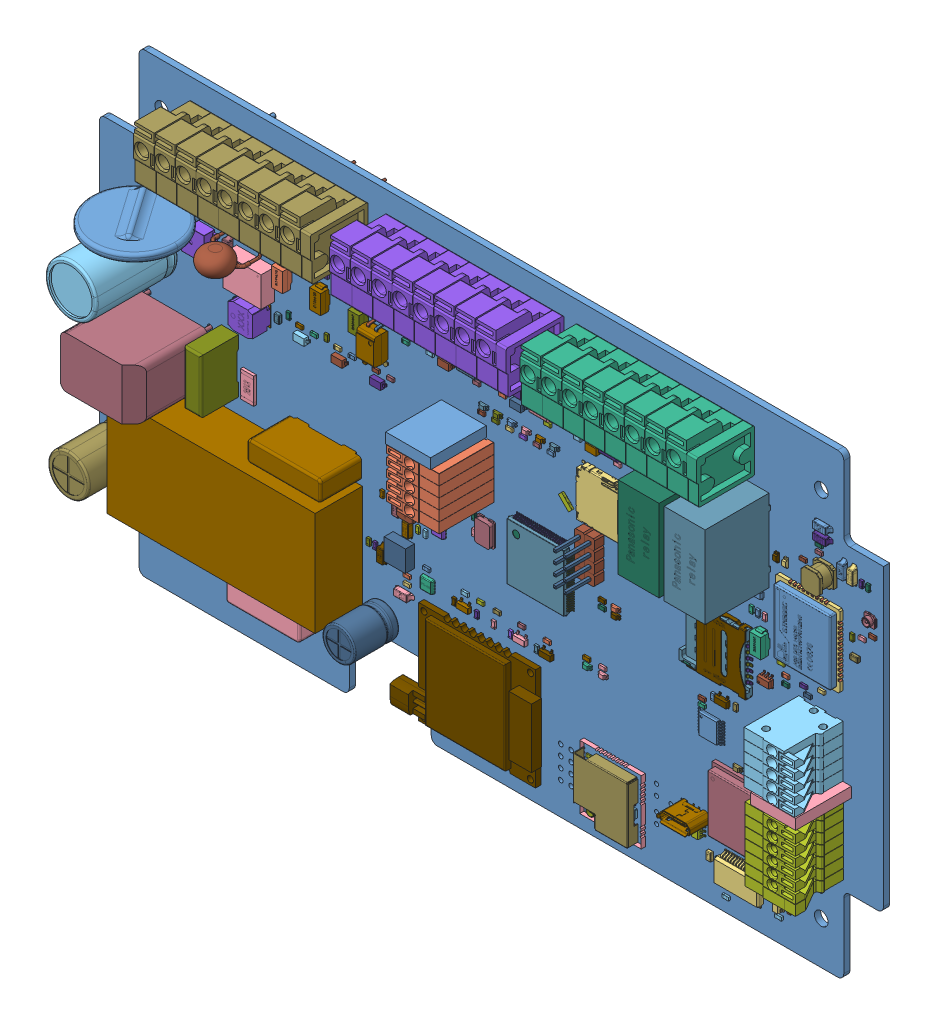
SolidWorks assembly Velvet_Controller_V1.2_2023, configuration Default. Lengths in mm. (continued)
Components (placement in the parent): (continued)
- Velvet_Controller_V1.2_2023(2)^Velvet_Controller_V1.2_2023-1: Velvet_Controller_V1.2_2023(2)^Velvet_Controller_V1.2_2023 [Default] at origin size (191.4 111.4 51.25) (virtual) (continued)
  - DD2lr^Velvet_Controller_V1.2_2023(2)_Velvet_Controller_V1.2_2023-1: DD2lr^Velvet_Controller_V1.2_2023(2)_Velvet_Controller_V1.2_2023 [Default] at origin size (15 15.75 3.52) (virtual) (continued)
    - 3D_RAK3172^DD2lr_Velvet_Controller_V1.2_2023(2)_Velvet_Controller_V1.2_2023-1: 3D_RAK3172^DD2lr_Velvet_Controller_V1.2_2023(2)_Velvet_Controller_V1.2_2023 [Default] at (133.2551 19.6 1) x (-1 0 0) z (0 0 1) size (15 15.75 3.52) (virtual) (continued)
      - C34^3D_RAK3172_DD2lr_Velvet_Controller_V1.2_2023(2)_Velvet_Controller_V1.2_2023-1: C34^3D_RAK3172_DD2lr_Velvet_Controller_V1.2_2023(2)_Velvet_Controller_V1.2_2023 [Default] at origin size (0.3 0.6 0.3) (virtual)
        - 0201_SMD_Capacitor^C34_3D_RAK3172_DD2lr_Velvet_Controller_V1.2_2023(2)_Velvet_Controller_V1.2_2023-1: 0201_SMD_Capacitor^C34_3D_RAK3172_DD2lr_Velvet_Controller_V1.2_2023(2)_Velvet_Controller_V1.2_2023 [Default] at (4.318 4.2211 0.2794) x (0 1 0) z (0 0 1) size (0.6 0.3 0.3) (virtual)
      - C35^3D_RAK3172_DD2lr_Velvet_Controller_V1.2_2023(2)_Velvet_Controller_V1.2_2023-1: C35^3D_RAK3172_DD2lr_Velvet_Controller_V1.2_2023(2)_Velvet_Controller_V1.2_2023 [Default] at origin size (0.6 0.3 0.3) (virtual)
        - 0201_SMD_Capacitor^C35_3D_RAK3172_DD2lr_Velvet_Controller_V1.2_2023(2)_Velvet_Controller_V1.2_2023-1: 0201_SMD_Capacitor^C35_3D_RAK3172_DD2lr_Velvet_Controller_V1.2_2023(2)_Velvet_Controller_V1.2_2023 [Default] at (9.0365 2.3622 0.2794) x (1 0 0) z (0 0 1) size (0.6 0.3 0.3) (virtual)
      - C36^3D_RAK3172_DD2lr_Velvet_Controller_V1.2_2023(2)_Velvet_Controller_V1.2_2023-1: C36^3D_RAK3172_DD2lr_Velvet_Controller_V1.2_2023(2)_Velvet_Controller_V1.2_2023 [Default] at origin size (0.3 0.6 0.3) (virtual)
        - 0201_SMD_Capacitor^C36_3D_RAK3172_DD2lr_Velvet_Controller_V1.2_2023(2)_Velvet_Controller_V1.2_2023-1: 0201_SMD_Capacitor^C36_3D_RAK3172_DD2lr_Velvet_Controller_V1.2_2023(2)_Velvet_Controller_V1.2_2023 [Default] at (13.0302 10.0751 0.2794) x (0 -1 0) z (0 0 1) size (0.6 0.3 0.3) (virtual)
      - C37^3D_RAK3172_DD2lr_Velvet_Controller_V1.2_2023(2)_Velvet_Controller_V1.2_2023-1: C37^3D_RAK3172_DD2lr_Velvet_Controller_V1.2_2023(2)_Velvet_Controller_V1.2_2023 [Default] at origin size (0.3 0.6 0.3) (virtual)
        - 0201_SMD_Capacitor^C37_3D_RAK3172_DD2lr_Velvet_Controller_V1.2_2023(2)_Velvet_Controller_V1.2_2023-1: 0201_SMD_Capacitor^C37_3D_RAK3172_DD2lr_Velvet_Controller_V1.2_2023(2)_Velvet_Controller_V1.2_2023 [Default] at (3.7338 4.2211 0.2794) x (0 1 0) z (0 0 1) size (0.6 0.3 0.3) (virtual)
      - C38^3D_RAK3172_DD2lr_Velvet_Controller_V1.2_2023(2)_Velvet_Controller_V1.2_2023-1: C38^3D_RAK3172_DD2lr_Velvet_Controller_V1.2_2023(2)_Velvet_Controller_V1.2_2023 [Default] at origin size (1 0.5 0.5) (virtual)
        - C0402^C38_3D_RAK3172_DD2lr_Velvet_Controller_V1.2_2023(2)_Velvet_Controller_V1.2_2023-1: C0402^C38_3D_RAK3172_DD2lr_Velvet_Controller_V1.2_2023(2)_Velvet_Controller_V1.2_2023 [Default] at (2.3114 4.7323 0.254) x (1 0 0) z (0 0 1) size (1 0.5 0.5) (virtual)
      - C39^3D_RAK3172_DD2lr_Velvet_Controller_V1.2_2023(2)_Velvet_Controller_V1.2_2023-1: C39^3D_RAK3172_DD2lr_Velvet_Controller_V1.2_2023(2)_Velvet_Controller_V1.2_2023 [Default] at origin size (0.6 0.3 0.3) (virtual)
        - 0201_SMD_Capacitor^C39_3D_RAK3172_DD2lr_Velvet_Controller_V1.2_2023(2)_Velvet_Controller_V1.2_2023-1: 0201_SMD_Capacitor^C39_3D_RAK3172_DD2lr_Velvet_Controller_V1.2_2023(2)_Velvet_Controller_V1.2_2023 [Default] at (4.0593 3.1881 0.2794) x (-1 0 0) z (0 0 1) size (0.6 0.3 0.3) (virtual)
      - C40^3D_RAK3172_DD2lr_Velvet_Controller_V1.2_2023(2)_Velvet_Controller_V1.2_2023-1: C40^3D_RAK3172_DD2lr_Velvet_Controller_V1.2_2023(2)_Velvet_Controller_V1.2_2023 [Default] at origin size (0.3 0.6 0.3) (virtual)
        - 0201_SMD_Capacitor^C40_3D_RAK3172_DD2lr_Velvet_Controller_V1.2_2023(2)_Velvet_Controller_V1.2_2023-1: 0201_SMD_Capacitor^C40_3D_RAK3172_DD2lr_Velvet_Controller_V1.2_2023(2)_Velvet_Controller_V1.2_2023 [Default] at (3.6576 1.7319 0.2794) x (0 1 0) z (0 0 1) size (0.6 0.3 0.3) (virtual)
      - L1^3D_RAK3172_DD2lr_Velvet_Controller_V1.2_2023(2)_Velvet_Controller_V1.2_2023-1: L1^3D_RAK3172_DD2lr_Velvet_Controller_V1.2_2023(2)_Velvet_Controller_V1.2_2023 [Default] at origin size (0.68 0.33 0.34) (virtual)
        - R0201^L1_3D_RAK3172_DD2lr_Velvet_Controller_V1.2_2023(2)_Velvet_Controller_V1.2_2023-1: R0201^L1_3D_RAK3172_DD2lr_Velvet_Controller_V1.2_2023(2)_Velvet_Controller_V1.2_2023 [Default] at (7.8526 11.2014 0) x (-1 0 0) z (0 1 0) size (0.68 0.34 0.33) (virtual)
      - L3^3D_RAK3172_DD2lr_Velvet_Controller_V1.2_2023(2)_Velvet_Controller_V1.2_2023-1: L3^3D_RAK3172_DD2lr_Velvet_Controller_V1.2_2023(2)_Velvet_Controller_V1.2_2023 [Default] at origin size (0.33 0.68 0.34) (virtual)
        - R0201^L3_3D_RAK3172_DD2lr_Velvet_Controller_V1.2_2023(2)_Velvet_Controller_V1.2_2023-1: R0201^L3_3D_RAK3172_DD2lr_Velvet_Controller_V1.2_2023(2)_Velvet_Controller_V1.2_2023 [Default] at (1.7272 13.1318 0) x (0 -1 0) z (-1 0 0) size (0.68 0.34 0.33) (virtual)
      - L5^3D_RAK3172_DD2lr_Velvet_Controller_V1.2_2023(2)_Velvet_Controller_V1.2_2023-1: L5^3D_RAK3172_DD2lr_Velvet_Controller_V1.2_2023(2)_Velvet_Controller_V1.2_2023 [Default] at origin size (0.68 0.33 0.34) (virtual)
        - R0201^L5_3D_RAK3172_DD2lr_Velvet_Controller_V1.2_2023(2)_Velvet_Controller_V1.2_2023-1: R0201^L5_3D_RAK3172_DD2lr_Velvet_Controller_V1.2_2023(2)_Velvet_Controller_V1.2_2023 [Default] at (8.0772 13.3096 0) x (-1 0 0) z (0 1 0) size (0.68 0.34 0.33) (virtual)
      - L6^3D_RAK3172_DD2lr_Velvet_Controller_V1.2_2023(2)_Velvet_Controller_V1.2_2023-1: L6^3D_RAK3172_DD2lr_Velvet_Controller_V1.2_2023(2)_Velvet_Controller_V1.2_2023 [Default] at origin size (1 0.5 0.5) (virtual)
        - C0402^L6_3D_RAK3172_DD2lr_Velvet_Controller_V1.2_2023(2)_Velvet_Controller_V1.2_2023-1: C0402^L6_3D_RAK3172_DD2lr_Velvet_Controller_V1.2_2023(2)_Velvet_Controller_V1.2_2023 [Default] at (5.822 11.0823 0.254) x (1 0 0) z (0 0 1) size (1 0.5 0.5) (virtual)
      - L7^3D_RAK3172_DD2lr_Velvet_Controller_V1.2_2023(2)_Velvet_Controller_V1.2_2023-1: L7^3D_RAK3172_DD2lr_Velvet_Controller_V1.2_2023(2)_Velvet_Controller_V1.2_2023 [Default] at origin size (0.68 0.33 0.34) (virtual)
        - R0201^L7_3D_RAK3172_DD2lr_Velvet_Controller_V1.2_2023(2)_Velvet_Controller_V1.2_2023-1: R0201^L7_3D_RAK3172_DD2lr_Velvet_Controller_V1.2_2023(2)_Velvet_Controller_V1.2_2023 [Default] at (3.5854 12.1158 0) x (1 0 0) z (0 -1 0) size (0.68 0.34 0.33) (virtual)
      - L9^3D_RAK3172_DD2lr_Velvet_Controller_V1.2_2023(2)_Velvet_Controller_V1.2_2023-1: L9^3D_RAK3172_DD2lr_Velvet_Controller_V1.2_2023(2)_Velvet_Controller_V1.2_2023 [Default] at origin size (1.15 0.55 0.41) (virtual)
        - RES_1005-0402^L9_3D_RAK3172_DD2lr_Velvet_Controller_V1.2_2023(2)_Velvet_Controller_V1.2_2023-1: RES_1005-0402^L9_3D_RAK3172_DD2lr_Velvet_Controller_V1.2_2023(2)_Velvet_Controller_V1.2_2023 [Default] at (3.9641 11.3538 0) x (-1 0 0) z (0 1 0) size (1.15 0.41 0.55) (virtual)
      - L20^3D_RAK3172_DD2lr_Velvet_Controller_V1.2_2023(2)_Velvet_Controller_V1.2_2023-1: L20^3D_RAK3172_DD2lr_Velvet_Controller_V1.2_2023(2)_Velvet_Controller_V1.2_2023 [Default] at origin size (1.6 0.8 0.3) (virtual)
        - 6559637360^L20_3D_RAK3172_DD2lr_Velvet_Controller_V1.2_2023(2)_Velvet_Controller_V1.2_2023-1: 6559637360^L20_3D_RAK3172_DD2lr_Velvet_Controller_V1.2_2023(2)_Velvet_Controller_V1.2_2023 [Default] at (12.3698 2.0828 0) x (-1 0 0) z (0 1 0) size (1.6 0.3 0.8) (virtual)
      - L30^3D_RAK3172_DD2lr_Velvet_Controller_V1.2_2023(2)_Velvet_Controller_V1.2_2023-1: L30^3D_RAK3172_DD2lr_Velvet_Controller_V1.2_2023(2)_Velvet_Controller_V1.2_2023 [Default] at origin size (1.15 0.55 0.41) (virtual)
        - RES_1005-0402^L30_3D_RAK3172_DD2lr_Velvet_Controller_V1.2_2023(2)_Velvet_Controller_V1.2_2023-1: RES_1005-0402^L30_3D_RAK3172_DD2lr_Velvet_Controller_V1.2_2023(2)_Velvet_Controller_V1.2_2023 [Default] at (7.1263 1.8 0) x (-1 0 0) z (0 1 0) size (1.15 0.41 0.55) (virtual)
      - X2^3D_RAK3172_DD2lr_Velvet_Controller_V1.2_2023(2)_Velvet_Controller_V1.2_2023-1: X2^3D_RAK3172_DD2lr_Velvet_Controller_V1.2_2023(2)_Velvet_Controller_V1.2_2023 [Default] at origin size (1.2 2 0.61) (virtual)
        - crystal_rtf2012^X2_3D_RAK3172_DD2lr_Velvet_Controller_V1.2_2023(2)_Velvet_Controller_V1.2_2023-1: crystal_rtf2012^X2_3D_RAK3172_DD2lr_Velvet_Controller_V1.2_2023(2)_Velvet_Controller_V1.2_2023 [Default] at (2.25 2.8402 0) x (0 1 0) z (1 0 0) size (2 0.61 1.2) (virtual)
      - R2^3D_RAK3172_DD2lr_Velvet_Controller_V1.2_2023(2)_Velvet_Controller_V1.2_2023-1: R2^3D_RAK3172_DD2lr_Velvet_Controller_V1.2_2023(2)_Velvet_Controller_V1.2_2023 [Default] at origin size (0.68 0.33 0.34) (virtual)
        - R0201^R2_3D_RAK3172_DD2lr_Velvet_Controller_V1.2_2023(2)_Velvet_Controller_V1.2_2023-1: R0201^R2_3D_RAK3172_DD2lr_Velvet_Controller_V1.2_2023(2)_Velvet_Controller_V1.2_2023 [Default] at (1.9613 10.1854 0) x (1 0 0) z (0 -1 0) size (0.68 0.34 0.33) (virtual)
      - C5^3D_RAK3172_DD2lr_Velvet_Controller_V1.2_2023(2)_Velvet_Controller_V1.2_2023-1: C5^3D_RAK3172_DD2lr_Velvet_Controller_V1.2_2023(2)_Velvet_Controller_V1.2_2023 [Default] at origin size (0.6 0.3 0.3) (virtual)
        - 0201_SMD_Capacitor^C5_3D_RAK3172_DD2lr_Velvet_Controller_V1.2_2023(2)_Velvet_Controller_V1.2_2023-1: 0201_SMD_Capacitor^C5_3D_RAK3172_DD2lr_Velvet_Controller_V1.2_2023(2)_Velvet_Controller_V1.2_2023 [Default] at (1.8749 6.9342 0.2794) x (-1 0 0) z (0 0 1) size (0.6 0.3 0.3) (virtual)
      - Free-Models^3D_RAK3172_DD2lr_Velvet_Controller_V1.2_2023(2)_Velvet_Controller_V1.2_2023-1: Free-Models^3D_RAK3172_DD2lr_Velvet_Controller_V1.2_2023(2)_Velvet_Controller_V1.2_2023 [Default] at origin size (13.4 13.9 2.5) (virtual)
        - D030A-________^Free-Models_3D_RAK3172_DD2lr_Velvet_Controller_V1.2_2023(2)_Velvet_Controller_V1.2_2023-1: D030A-________^Free-Models_3D_RAK3172_DD2lr_Velvet_Controller_V1.2_2023(2)_Velvet_Controller_V1.2_2023 [Default] at (2.429 -1.8288 0) size (13.4 13.9 2.5) (virtual)
  - DD1wf^Velvet_Controller_V1.2_2023(2)_Velvet_Controller_V1.2_2023-1: DD1wf^Velvet_Controller_V1.2_2023(2)_Velvet_Controller_V1.2_2023 [Default] at origin size (15.4 15.4 2.55) (virtual)
    - 6168615376^DD1wf_Velvet_Controller_V1.2_2023(2)_Velvet_Controller_V1.2_2023-1: 6168615376^DD1wf_Velvet_Controller_V1.2_2023(2)_Velvet_Controller_V1.2_2023 [Default] at (158.15 23.5 0) x (0 -1 0) z (-1 0 0) size (15.4 2.55 15.4) (virtual)
  - DD1mc^Velvet_Controller_V1.2_2023(2)_Velvet_Controller_V1.2_2023-1: DD1mc^Velvet_Controller_V1.2_2023(2)_Velvet_Controller_V1.2_2023 [Default] at origin size (16 16 1.6) (virtual)
    - 6168610096^DD1mc_Velvet_Controller_V1.2_2023(2)_Velvet_Controller_V1.2_2023-1: 6168610096^DD1mc_Velvet_Controller_V1.2_2023(2)_Velvet_Controller_V1.2_2023 [Default] at (108 51.3 0) x (1 0 0) z (0 0 1) size (16 16 1.6) (virtual)
      - Body-4^6168610096_DD1mc_Velvet_Controller_V1.2_2023(2)_Velvet_Controller_V1.2_2023-1: Body-4^6168610096_DD1mc_Velvet_Controller_V1.2_2023(2)_Velvet_Controller_V1.2_2023 [Default] at (-7 -7 0) size (14.01 14.01 1.45) (virtual)
        - Open CASCADE STEP translator 7.5 4.2.1^Body-4_6168610096_DD1mc_Velvet_Controller_V1.2_2023(2)_Velvet_Controller_V1.2_2023-1: Open CASCADE STEP translator 7.5 4.2.1^Body-4_6168610096_DD1mc_Velvet_Controller_V1.2_2023(2)_Velvet_Controller_V1.2_2023 [Default] at origin size (14.01 14.01 1.45) (virtual)
      - Open CASCADE STEP translator 7.5 4.1^6168610096_DD1mc_Velvet_Controller_V1.2_2023(2)_Velvet_Controller_V1.2_2023-1: Open CASCADE STEP translator 7.5 4.1^6168610096_DD1mc_Velvet_Controller_V1.2_2023(2)_Velvet_Controller_V1.2_2023 [Default] at (-7 -7 0.001) size (1.76 1.76 0.01) (virtual)
      - Leader^6168610096_DD1mc_Velvet_Controller_V1.2_2023(2)_Velvet_Controller_V1.2_2023-1: Leader^6168610096_DD1mc_Velvet_Controller_V1.2_2023(2)_Velvet_Controller_V1.2_2023 [Default] at (-7 -6 0) x (-1 0 0) z (0 0 1) size (1 0.22 0.93) (virtual)
      - Leader^6168610096_DD1mc_Velvet_Controller_V1.2_2023(2)_Velvet_Controller_V1.2_2023-2: Leader^6168610096_DD1mc_Velvet_Controller_V1.2_2023(2)_Velvet_Controller_V1.2_2023 [Default] at (-7 -5.5 0) x (-1 0 0) z (0 0 1) size (1 0.22 0.93) (virtual)
      - Leader^6168610096_DD1mc_Velvet_Controller_V1.2_2023(2)_Velvet_Controller_V1.2_2023-3: Leader^6168610096_DD1mc_Velvet_Controller_V1.2_2023(2)_Velvet_Controller_V1.2_2023 [Default] at (-7 -5 0) x (-1 0 0) z (0 0 1) size (1 0.22 0.93) (virtual)
      - Leader^6168610096_DD1mc_Velvet_Controller_V1.2_2023(2)_Velvet_Controller_V1.2_2023-4: Leader^6168610096_DD1mc_Velvet_Controller_V1.2_2023(2)_Velvet_Controller_V1.2_2023 [Default] at (-7 -4.5 0) x (-1 0 0) z (0 0 1) size (1 0.22 0.93) (virtual)
      - Leader^6168610096_DD1mc_Velvet_Controller_V1.2_2023(2)_Velvet_Controller_V1.2_2023-5: Leader^6168610096_DD1mc_Velvet_Controller_V1.2_2023(2)_Velvet_Controller_V1.2_2023 [Default] at (-7 -4 0) x (-1 0 0) z (0 0 1) size (1 0.22 0.93) (virtual)
      - Leader^6168610096_DD1mc_Velvet_Controller_V1.2_2023(2)_Velvet_Controller_V1.2_2023-6: Leader^6168610096_DD1mc_Velvet_Controller_V1.2_2023(2)_Velvet_Controller_V1.2_2023 [Default] at (-7 -3.5 0) x (-1 0 0) z (0 0 1) size (1 0.22 0.93) (virtual)
      - Leader^6168610096_DD1mc_Velvet_Controller_V1.2_2023(2)_Velvet_Controller_V1.2_2023-7: Leader^6168610096_DD1mc_Velvet_Controller_V1.2_2023(2)_Velvet_Controller_V1.2_2023 [Default] at (-7 -3 0) x (-1 0 0) z (0 0 1) size (1 0.22 0.93) (virtual)
      - Leader^6168610096_DD1mc_Velvet_Controller_V1.2_2023(2)_Velvet_Controller_V1.2_2023-8: Leader^6168610096_DD1mc_Velvet_Controller_V1.2_2023(2)_Velvet_Controller_V1.2_2023 [Default] at (-7 -2.5 0) x (-1 0 0) z (0 0 1) size (1 0.22 0.93) (virtual)
      - Leader^6168610096_DD1mc_Velvet_Controller_V1.2_2023(2)_Velvet_Controller_V1.2_2023-9: Leader^6168610096_DD1mc_Velvet_Controller_V1.2_2023(2)_Velvet_Controller_V1.2_2023 [Default] at (-7 -2 0) x (-1 0 0) z (0 0 1) size (1 0.22 0.93) (virtual)
      - Leader^6168610096_DD1mc_Velvet_Controller_V1.2_2023(2)_Velvet_Controller_V1.2_2023-10: Leader^6168610096_DD1mc_Velvet_Controller_V1.2_2023(2)_Velvet_Controller_V1.2_2023 [Default] at (-7 -1.5 0) x (-1 0 0) z (0 0 1) size (1 0.22 0.93) (virtual)
      - Leader^6168610096_DD1mc_Velvet_Controller_V1.2_2023(2)_Velvet_Controller_V1.2_2023-11: Leader^6168610096_DD1mc_Velvet_Controller_V1.2_2023(2)_Velvet_Controller_V1.2_2023 [Default] at (-7 -1 0) x (-1 0 0) z (0 0 1) size (1 0.22 0.93) (virtual)
      - Leader^6168610096_DD1mc_Velvet_Controller_V1.2_2023(2)_Velvet_Controller_V1.2_2023-12: Leader^6168610096_DD1mc_Velvet_Controller_V1.2_2023(2)_Velvet_Controller_V1.2_2023 [Default] at (-7 -0.5 0) x (-1 0 0) z (0 0 1) size (1 0.22 0.93) (virtual)
      - Leader^6168610096_DD1mc_Velvet_Controller_V1.2_2023(2)_Velvet_Controller_V1.2_2023-13: Leader^6168610096_DD1mc_Velvet_Controller_V1.2_2023(2)_Velvet_Controller_V1.2_2023 [Default] at (-7 0 0) x (-1 0 0) z (0 0 1) size (1 0.22 0.93) (virtual)
      - Leader^6168610096_DD1mc_Velvet_Controller_V1.2_2023(2)_Velvet_Controller_V1.2_2023-14: Leader^6168610096_DD1mc_Velvet_Controller_V1.2_2023(2)_Velvet_Controller_V1.2_2023 [Default] at (-7 0.5 0) x (-1 0 0) z (0 0 1) size (1 0.22 0.93) (virtual)
      - Leader^6168610096_DD1mc_Velvet_Controller_V1.2_2023(2)_Velvet_Controller_V1.2_2023-15: Leader^6168610096_DD1mc_Velvet_Controller_V1.2_2023(2)_Velvet_Controller_V1.2_2023 [Default] at (-7 1 0) x (-1 0 0) z (0 0 1) size (1 0.22 0.93) (virtual)
      - Leader^6168610096_DD1mc_Velvet_Controller_V1.2_2023(2)_Velvet_Controller_V1.2_2023-16: Leader^6168610096_DD1mc_Velvet_Controller_V1.2_2023(2)_Velvet_Controller_V1.2_2023 [Default] at (-7 1.5 0) x (-1 0 0) z (0 0 1) size (1 0.22 0.93) (virtual)
      - Leader^6168610096_DD1mc_Velvet_Controller_V1.2_2023(2)_Velvet_Controller_V1.2_2023-17: Leader^6168610096_DD1mc_Velvet_Controller_V1.2_2023(2)_Velvet_Controller_V1.2_2023 [Default] at (-7 2 0) x (-1 0 0) z (0 0 1) size (1 0.22 0.93) (virtual)
      - Leader^6168610096_DD1mc_Velvet_Controller_V1.2_2023(2)_Velvet_Controller_V1.2_2023-18: Leader^6168610096_DD1mc_Velvet_Controller_V1.2_2023(2)_Velvet_Controller_V1.2_2023 [Default] at (-7 2.5 0) x (-1 0 0) z (0 0 1) size (1 0.22 0.93) (virtual)
      - Leader^6168610096_DD1mc_Velvet_Controller_V1.2_2023(2)_Velvet_Controller_V1.2_2023-19: Leader^6168610096_DD1mc_Velvet_Controller_V1.2_2023(2)_Velvet_Controller_V1.2_2023 [Default] at (-7 3 0) x (-1 0 0) z (0 0 1) size (1 0.22 0.93) (virtual)
      - Leader^6168610096_DD1mc_Velvet_Controller_V1.2_2023(2)_Velvet_Controller_V1.2_2023-20: Leader^6168610096_DD1mc_Velvet_Controller_V1.2_2023(2)_Velvet_Controller_V1.2_2023 [Default] at (-7 3.5 0) x (-1 0 0) z (0 0 1) size (1 0.22 0.93) (virtual)
      - Leader^6168610096_DD1mc_Velvet_Controller_V1.2_2023(2)_Velvet_Controller_V1.2_2023-21: Leader^6168610096_DD1mc_Velvet_Controller_V1.2_2023(2)_Velvet_Controller_V1.2_2023 [Default] at (-7 4 0) x (-1 0 0) z (0 0 1) size (1 0.22 0.93) (virtual)
      - Leader^6168610096_DD1mc_Velvet_Controller_V1.2_2023(2)_Velvet_Controller_V1.2_2023-22: Leader^6168610096_DD1mc_Velvet_Controller_V1.2_2023(2)_Velvet_Controller_V1.2_2023 [Default] at (-7 4.5 0) x (-1 0 0) z (0 0 1) size (1 0.22 0.93) (virtual)
      - Leader^6168610096_DD1mc_Velvet_Controller_V1.2_2023(2)_Velvet_Controller_V1.2_2023-23: Leader^6168610096_DD1mc_Velvet_Controller_V1.2_2023(2)_Velvet_Controller_V1.2_2023 [Default] at (-7 5 0) x (-1 0 0) z (0 0 1) size (1 0.22 0.93) (virtual)
      - Leader^6168610096_DD1mc_Velvet_Controller_V1.2_2023(2)_Velvet_Controller_V1.2_2023-24: Leader^6168610096_DD1mc_Velvet_Controller_V1.2_2023(2)_Velvet_Controller_V1.2_2023 [Default] at (-7 5.5 0) x (-1 0 0) z (0 0 1) size (1 0.22 0.93) (virtual)
      - Leader^6168610096_DD1mc_Velvet_Controller_V1.2_2023(2)_Velvet_Controller_V1.2_2023-25: Leader^6168610096_DD1mc_Velvet_Controller_V1.2_2023(2)_Velvet_Controller_V1.2_2023 [Default] at (-7 6 0) x (-1 0 0) z (0 0 1) size (1 0.22 0.93) (virtual)
      - Leader^6168610096_DD1mc_Velvet_Controller_V1.2_2023(2)_Velvet_Controller_V1.2_2023-26: Leader^6168610096_DD1mc_Velvet_Controller_V1.2_2023(2)_Velvet_Controller_V1.2_2023 [Default] at (7 -6 0) size (1 0.22 0.93) (virtual)
      - Leader^6168610096_DD1mc_Velvet_Controller_V1.2_2023(2)_Velvet_Controller_V1.2_2023-27: Leader^6168610096_DD1mc_Velvet_Controller_V1.2_2023(2)_Velvet_Controller_V1.2_2023 [Default] at (7 -5.5 0) size (1 0.22 0.93) (virtual)
      - Leader^6168610096_DD1mc_Velvet_Controller_V1.2_2023(2)_Velvet_Controller_V1.2_2023-28: Leader^6168610096_DD1mc_Velvet_Controller_V1.2_2023(2)_Velvet_Controller_V1.2_2023 [Default] at (7 -5 0) size (1 0.22 0.93) (virtual)
      - Leader^6168610096_DD1mc_Velvet_Controller_V1.2_2023(2)_Velvet_Controller_V1.2_2023-29: Leader^6168610096_DD1mc_Velvet_Controller_V1.2_2023(2)_Velvet_Controller_V1.2_2023 [Default] at (7 -4.5 0) size (1 0.22 0.93) (virtual)
      - Leader^6168610096_DD1mc_Velvet_Controller_V1.2_2023(2)_Velvet_Controller_V1.2_2023-30: Leader^6168610096_DD1mc_Velvet_Controller_V1.2_2023(2)_Velvet_Controller_V1.2_2023 [Default] at (7 -4 0) size (1 0.22 0.93) (virtual)
      - Leader^6168610096_DD1mc_Velvet_Controller_V1.2_2023(2)_Velvet_Controller_V1.2_2023-31: Leader^6168610096_DD1mc_Velvet_Controller_V1.2_2023(2)_Velvet_Controller_V1.2_2023 [Default] at (7 -3.5 0) size (1 0.22 0.93) (virtual)
      - Leader^6168610096_DD1mc_Velvet_Controller_V1.2_2023(2)_Velvet_Controller_V1.2_2023-32: Leader^6168610096_DD1mc_Velvet_Controller_V1.2_2023(2)_Velvet_Controller_V1.2_2023 [Default] at (7 -3 0) size (1 0.22 0.93) (virtual)
      - Leader^6168610096_DD1mc_Velvet_Controller_V1.2_2023(2)_Velvet_Controller_V1.2_2023-33: Leader^6168610096_DD1mc_Velvet_Controller_V1.2_2023(2)_Velvet_Controller_V1.2_2023 [Default] at (7 -2.5 0) size (1 0.22 0.93) (virtual)
      - Leader^6168610096_DD1mc_Velvet_Controller_V1.2_2023(2)_Velvet_Controller_V1.2_2023-34: Leader^6168610096_DD1mc_Velvet_Controller_V1.2_2023(2)_Velvet_Controller_V1.2_2023 [Default] at (7 -2 0) size (1 0.22 0.93) (virtual)
      - Leader^6168610096_DD1mc_Velvet_Controller_V1.2_2023(2)_Velvet_Controller_V1.2_2023-35: Leader^6168610096_DD1mc_Velvet_Controller_V1.2_2023(2)_Velvet_Controller_V1.2_2023 [Default] at (7 -1.5 0) size (1 0.22 0.93) (virtual)
      - Leader^6168610096_DD1mc_Velvet_Controller_V1.2_2023(2)_Velvet_Controller_V1.2_2023-36: Leader^6168610096_DD1mc_Velvet_Controller_V1.2_2023(2)_Velvet_Controller_V1.2_2023 [Default] at (7 -1 0) size (1 0.22 0.93) (virtual)
      - Leader^6168610096_DD1mc_Velvet_Controller_V1.2_2023(2)_Velvet_Controller_V1.2_2023-37: Leader^6168610096_DD1mc_Velvet_Controller_V1.2_2023(2)_Velvet_Controller_V1.2_2023 [Default] at (7 -0.5 0) size (1 0.22 0.93) (virtual)
      - Leader^6168610096_DD1mc_Velvet_Controller_V1.2_2023(2)_Velvet_Controller_V1.2_2023-38: Leader^6168610096_DD1mc_Velvet_Controller_V1.2_2023(2)_Velvet_Controller_V1.2_2023 [Default] at (7 0 0) size (1 0.22 0.93) (virtual)
      - Leader^6168610096_DD1mc_Velvet_Controller_V1.2_2023(2)_Velvet_Controller_V1.2_2023-39: Leader^6168610096_DD1mc_Velvet_Controller_V1.2_2023(2)_Velvet_Controller_V1.2_2023 [Default] at (7 0.5 0) size (1 0.22 0.93) (virtual)
      - Leader^6168610096_DD1mc_Velvet_Controller_V1.2_2023(2)_Velvet_Controller_V1.2_2023-40: Leader^6168610096_DD1mc_Velvet_Controller_V1.2_2023(2)_Velvet_Controller_V1.2_2023 [Default] at (7 1 0) size (1 0.22 0.93) (virtual)
      - Leader^6168610096_DD1mc_Velvet_Controller_V1.2_2023(2)_Velvet_Controller_V1.2_2023-41: Leader^6168610096_DD1mc_Velvet_Controller_V1.2_2023(2)_Velvet_Controller_V1.2_2023 [Default] at (7 1.5 0) size (1 0.22 0.93) (virtual)
      - Leader^6168610096_DD1mc_Velvet_Controller_V1.2_2023(2)_Velvet_Controller_V1.2_2023-42: Leader^6168610096_DD1mc_Velvet_Controller_V1.2_2023(2)_Velvet_Controller_V1.2_2023 [Default] at (7 2 0) size (1 0.22 0.93) (virtual)
      - Leader^6168610096_DD1mc_Velvet_Controller_V1.2_2023(2)_Velvet_Controller_V1.2_2023-43: Leader^6168610096_DD1mc_Velvet_Controller_V1.2_2023(2)_Velvet_Controller_V1.2_2023 [Default] at (7 2.5 0) size (1 0.22 0.93) (virtual)
      - Leader^6168610096_DD1mc_Velvet_Controller_V1.2_2023(2)_Velvet_Controller_V1.2_2023-44: Leader^6168610096_DD1mc_Velvet_Controller_V1.2_2023(2)_Velvet_Controller_V1.2_2023 [Default] at (7 3 0) size (1 0.22 0.93) (virtual)
      - Leader^6168610096_DD1mc_Velvet_Controller_V1.2_2023(2)_Velvet_Controller_V1.2_2023-45: Leader^6168610096_DD1mc_Velvet_Controller_V1.2_2023(2)_Velvet_Controller_V1.2_2023 [Default] at (7 3.5 0) size (1 0.22 0.93) (virtual)
      - Leader^6168610096_DD1mc_Velvet_Controller_V1.2_2023(2)_Velvet_Controller_V1.2_2023-46: Leader^6168610096_DD1mc_Velvet_Controller_V1.2_2023(2)_Velvet_Controller_V1.2_2023 [Default] at (7 4 0) size (1 0.22 0.93) (virtual)
      - Leader^6168610096_DD1mc_Velvet_Controller_V1.2_2023(2)_Velvet_Controller_V1.2_2023-47: Leader^6168610096_DD1mc_Velvet_Controller_V1.2_2023(2)_Velvet_Controller_V1.2_2023 [Default] at (7 4.5 0) size (1 0.22 0.93) (virtual)
      - Leader^6168610096_DD1mc_Velvet_Controller_V1.2_2023(2)_Velvet_Controller_V1.2_2023-48: Leader^6168610096_DD1mc_Velvet_Controller_V1.2_2023(2)_Velvet_Controller_V1.2_2023 [Default] at (7 5 0) size (1 0.22 0.93) (virtual)
      - Leader^6168610096_DD1mc_Velvet_Controller_V1.2_2023(2)_Velvet_Controller_V1.2_2023-49: Leader^6168610096_DD1mc_Velvet_Controller_V1.2_2023(2)_Velvet_Controller_V1.2_2023 [Default] at (7 5.5 0) size (1 0.22 0.93) (virtual)
      - Leader^6168610096_DD1mc_Velvet_Controller_V1.2_2023(2)_Velvet_Controller_V1.2_2023-50: Leader^6168610096_DD1mc_Velvet_Controller_V1.2_2023(2)_Velvet_Controller_V1.2_2023 [Default] at (7 6 0) size (1 0.22 0.93) (virtual)
      - Leader-5^6168610096_DD1mc_Velvet_Controller_V1.2_2023(2)_Velvet_Controller_V1.2_2023-1: Leader-5^6168610096_DD1mc_Velvet_Controller_V1.2_2023(2)_Velvet_Controller_V1.2_2023 [Default] at (-6 -7 0) x (0 -1 0) z (0 0 1) size (1 0.22 0.93) (virtual)
      - Leader-5^6168610096_DD1mc_Velvet_Controller_V1.2_2023(2)_Velvet_Controller_V1.2_2023-2: Leader-5^6168610096_DD1mc_Velvet_Controller_V1.2_2023(2)_Velvet_Controller_V1.2_2023 [Default] at (-5.5 -7 0) x (0 -1 0) z (0 0 1) size (1 0.22 0.93) (virtual)
      - Leader-5^6168610096_DD1mc_Velvet_Controller_V1.2_2023(2)_Velvet_Controller_V1.2_2023-3: Leader-5^6168610096_DD1mc_Velvet_Controller_V1.2_2023(2)_Velvet_Controller_V1.2_2023 [Default] at (-5 -7 0) x (0 -1 0) z (0 0 1) size (1 0.22 0.93) (virtual)
      - Leader-5^6168610096_DD1mc_Velvet_Controller_V1.2_2023(2)_Velvet_Controller_V1.2_2023-4: Leader-5^6168610096_DD1mc_Velvet_Controller_V1.2_2023(2)_Velvet_Controller_V1.2_2023 [Default] at (-4.5 -7 0) x (0 -1 0) z (0 0 1) size (1 0.22 0.93) (virtual)
      - Leader-5^6168610096_DD1mc_Velvet_Controller_V1.2_2023(2)_Velvet_Controller_V1.2_2023-5: Leader-5^6168610096_DD1mc_Velvet_Controller_V1.2_2023(2)_Velvet_Controller_V1.2_2023 [Default] at (-4 -7 0) x (0 -1 0) z (0 0 1) size (1 0.22 0.93) (virtual)
      - Leader-5^6168610096_DD1mc_Velvet_Controller_V1.2_2023(2)_Velvet_Controller_V1.2_2023-6: Leader-5^6168610096_DD1mc_Velvet_Controller_V1.2_2023(2)_Velvet_Controller_V1.2_2023 [Default] at (-3.5 -7 0) x (0 -1 0) z (0 0 1) size (1 0.22 0.93) (virtual)
      - Leader-5^6168610096_DD1mc_Velvet_Controller_V1.2_2023(2)_Velvet_Controller_V1.2_2023-7: Leader-5^6168610096_DD1mc_Velvet_Controller_V1.2_2023(2)_Velvet_Controller_V1.2_2023 [Default] at (-3 -7 0) x (0 -1 0) z (0 0 1) size (1 0.22 0.93) (virtual)
      - Leader-5^6168610096_DD1mc_Velvet_Controller_V1.2_2023(2)_Velvet_Controller_V1.2_2023-8: Leader-5^6168610096_DD1mc_Velvet_Controller_V1.2_2023(2)_Velvet_Controller_V1.2_2023 [Default] at (-2.5 -7 0) x (0 -1 0) z (0 0 1) size (1 0.22 0.93) (virtual)
      - Leader-5^6168610096_DD1mc_Velvet_Controller_V1.2_2023(2)_Velvet_Controller_V1.2_2023-9: Leader-5^6168610096_DD1mc_Velvet_Controller_V1.2_2023(2)_Velvet_Controller_V1.2_2023 [Default] at (-2 -7 0) x (0 -1 0) z (0 0 1) size (1 0.22 0.93) (virtual)
      - Leader-5^6168610096_DD1mc_Velvet_Controller_V1.2_2023(2)_Velvet_Controller_V1.2_2023-10: Leader-5^6168610096_DD1mc_Velvet_Controller_V1.2_2023(2)_Velvet_Controller_V1.2_2023 [Default] at (-1.5 -7 0) x (0 -1 0) z (0 0 1) size (1 0.22 0.93) (virtual)
      - Leader-5^6168610096_DD1mc_Velvet_Controller_V1.2_2023(2)_Velvet_Controller_V1.2_2023-11: Leader-5^6168610096_DD1mc_Velvet_Controller_V1.2_2023(2)_Velvet_Controller_V1.2_2023 [Default] at (-1 -7 0) x (0 -1 0) z (0 0 1) size (1 0.22 0.93) (virtual)
      - Leader-5^6168610096_DD1mc_Velvet_Controller_V1.2_2023(2)_Velvet_Controller_V1.2_2023-12: Leader-5^6168610096_DD1mc_Velvet_Controller_V1.2_2023(2)_Velvet_Controller_V1.2_2023 [Default] at (-0.5 -7 0) x (0 -1 0) z (0 0 1) size (1 0.22 0.93) (virtual)
      - Leader-5^6168610096_DD1mc_Velvet_Controller_V1.2_2023(2)_Velvet_Controller_V1.2_2023-13: Leader-5^6168610096_DD1mc_Velvet_Controller_V1.2_2023(2)_Velvet_Controller_V1.2_2023 [Default] at (0 -7 0) x (0 -1 0) z (0 0 1) size (1 0.22 0.93) (virtual)
      - Leader-5^6168610096_DD1mc_Velvet_Controller_V1.2_2023(2)_Velvet_Controller_V1.2_2023-14: Leader-5^6168610096_DD1mc_Velvet_Controller_V1.2_2023(2)_Velvet_Controller_V1.2_2023 [Default] at (0.5 -7 0) x (0 -1 0) z (0 0 1) size (1 0.22 0.93) (virtual)
      - Leader-5^6168610096_DD1mc_Velvet_Controller_V1.2_2023(2)_Velvet_Controller_V1.2_2023-15: Leader-5^6168610096_DD1mc_Velvet_Controller_V1.2_2023(2)_Velvet_Controller_V1.2_2023 [Default] at (1 -7 0) x (0 -1 0) z (0 0 1) size (1 0.22 0.93) (virtual)
      - Leader-5^6168610096_DD1mc_Velvet_Controller_V1.2_2023(2)_Velvet_Controller_V1.2_2023-16: Leader-5^6168610096_DD1mc_Velvet_Controller_V1.2_2023(2)_Velvet_Controller_V1.2_2023 [Default] at (1.5 -7 0) x (0 -1 0) z (0 0 1) size (1 0.22 0.93) (virtual)
      - Leader-5^6168610096_DD1mc_Velvet_Controller_V1.2_2023(2)_Velvet_Controller_V1.2_2023-17: Leader-5^6168610096_DD1mc_Velvet_Controller_V1.2_2023(2)_Velvet_Controller_V1.2_2023 [Default] at (2 -7 0) x (0 -1 0) z (0 0 1) size (1 0.22 0.93) (virtual)
      - Leader-5^6168610096_DD1mc_Velvet_Controller_V1.2_2023(2)_Velvet_Controller_V1.2_2023-18: Leader-5^6168610096_DD1mc_Velvet_Controller_V1.2_2023(2)_Velvet_Controller_V1.2_2023 [Default] at (2.5 -7 0) x (0 -1 0) z (0 0 1) size (1 0.22 0.93) (virtual)
      - Leader-5^6168610096_DD1mc_Velvet_Controller_V1.2_2023(2)_Velvet_Controller_V1.2_2023-19: Leader-5^6168610096_DD1mc_Velvet_Controller_V1.2_2023(2)_Velvet_Controller_V1.2_2023 [Default] at (3 -7 0) x (0 -1 0) z (0 0 1) size (1 0.22 0.93) (virtual)
      - Leader-5^6168610096_DD1mc_Velvet_Controller_V1.2_2023(2)_Velvet_Controller_V1.2_2023-20: Leader-5^6168610096_DD1mc_Velvet_Controller_V1.2_2023(2)_Velvet_Controller_V1.2_2023 [Default] at (3.5 -7 0) x (0 -1 0) z (0 0 1) size (1 0.22 0.93) (virtual)
      - Leader-5^6168610096_DD1mc_Velvet_Controller_V1.2_2023(2)_Velvet_Controller_V1.2_2023-21: Leader-5^6168610096_DD1mc_Velvet_Controller_V1.2_2023(2)_Velvet_Controller_V1.2_2023 [Default] at (4 -7 0) x (0 -1 0) z (0 0 1) size (1 0.22 0.93) (virtual)
      - Leader-5^6168610096_DD1mc_Velvet_Controller_V1.2_2023(2)_Velvet_Controller_V1.2_2023-22: Leader-5^6168610096_DD1mc_Velvet_Controller_V1.2_2023(2)_Velvet_Controller_V1.2_2023 [Default] at (4.5 -7 0) x (0 -1 0) z (0 0 1) size (1 0.22 0.93) (virtual)
      - Leader-5^6168610096_DD1mc_Velvet_Controller_V1.2_2023(2)_Velvet_Controller_V1.2_2023-23: Leader-5^6168610096_DD1mc_Velvet_Controller_V1.2_2023(2)_Velvet_Controller_V1.2_2023 [Default] at (5 -7 0) x (0 -1 0) z (0 0 1) size (1 0.22 0.93) (virtual)
      - Leader-5^6168610096_DD1mc_Velvet_Controller_V1.2_2023(2)_Velvet_Controller_V1.2_2023-24: Leader-5^6168610096_DD1mc_Velvet_Controller_V1.2_2023(2)_Velvet_Controller_V1.2_2023 [Default] at (5.5 -7 0) x (0 -1 0) z (0 0 1) size (1 0.22 0.93) (virtual)
      - Leader-5^6168610096_DD1mc_Velvet_Controller_V1.2_2023(2)_Velvet_Controller_V1.2_2023-25: Leader-5^6168610096_DD1mc_Velvet_Controller_V1.2_2023(2)_Velvet_Controller_V1.2_2023 [Default] at (6 -7 0) x (0 -1 0) z (0 0 1) size (1 0.22 0.93) (virtual)
      - Leader-5^6168610096_DD1mc_Velvet_Controller_V1.2_2023(2)_Velvet_Controller_V1.2_2023-26: Leader-5^6168610096_DD1mc_Velvet_Controller_V1.2_2023(2)_Velvet_Controller_V1.2_2023 [Default] at (-6 7 0) x (0 1 0) z (0 0 1) size (1 0.22 0.93) (virtual)
      - Leader-5^6168610096_DD1mc_Velvet_Controller_V1.2_2023(2)_Velvet_Controller_V1.2_2023-27: Leader-5^6168610096_DD1mc_Velvet_Controller_V1.2_2023(2)_Velvet_Controller_V1.2_2023 [Default] at (-5.5 7 0) x (0 1 0) z (0 0 1) size (1 0.22 0.93) (virtual)
      - Leader-5^6168610096_DD1mc_Velvet_Controller_V1.2_2023(2)_Velvet_Controller_V1.2_2023-28: Leader-5^6168610096_DD1mc_Velvet_Controller_V1.2_2023(2)_Velvet_Controller_V1.2_2023 [Default] at (-5 7 0) x (0 1 0) z (0 0 1) size (1 0.22 0.93) (virtual)
      - Leader-5^6168610096_DD1mc_Velvet_Controller_V1.2_2023(2)_Velvet_Controller_V1.2_2023-29: Leader-5^6168610096_DD1mc_Velvet_Controller_V1.2_2023(2)_Velvet_Controller_V1.2_2023 [Default] at (-4.5 7 0) x (0 1 0) z (0 0 1) size (1 0.22 0.93) (virtual)
      - Leader-5^6168610096_DD1mc_Velvet_Controller_V1.2_2023(2)_Velvet_Controller_V1.2_2023-30: Leader-5^6168610096_DD1mc_Velvet_Controller_V1.2_2023(2)_Velvet_Controller_V1.2_2023 [Default] at (-4 7 0) x (0 1 0) z (0 0 1) size (1 0.22 0.93) (virtual)
      - Leader-5^6168610096_DD1mc_Velvet_Controller_V1.2_2023(2)_Velvet_Controller_V1.2_2023-31: Leader-5^6168610096_DD1mc_Velvet_Controller_V1.2_2023(2)_Velvet_Controller_V1.2_2023 [Default] at (-3.5 7 0) x (0 1 0) z (0 0 1) size (1 0.22 0.93) (virtual)
      - Leader-5^6168610096_DD1mc_Velvet_Controller_V1.2_2023(2)_Velvet_Controller_V1.2_2023-32: Leader-5^6168610096_DD1mc_Velvet_Controller_V1.2_2023(2)_Velvet_Controller_V1.2_2023 [Default] at (-3 7 0) x (0 1 0) z (0 0 1) size (1 0.22 0.93) (virtual)
      - Leader-5^6168610096_DD1mc_Velvet_Controller_V1.2_2023(2)_Velvet_Controller_V1.2_2023-33: Leader-5^6168610096_DD1mc_Velvet_Controller_V1.2_2023(2)_Velvet_Controller_V1.2_2023 [Default] at (-2.5 7 0) x (0 1 0) z (0 0 1) size (1 0.22 0.93) (virtual)
      - Leader-5^6168610096_DD1mc_Velvet_Controller_V1.2_2023(2)_Velvet_Controller_V1.2_2023-34: Leader-5^6168610096_DD1mc_Velvet_Controller_V1.2_2023(2)_Velvet_Controller_V1.2_2023 [Default] at (-2 7 0) x (0 1 0) z (0 0 1) size (1 0.22 0.93) (virtual)
      - Leader-5^6168610096_DD1mc_Velvet_Controller_V1.2_2023(2)_Velvet_Controller_V1.2_2023-35: Leader-5^6168610096_DD1mc_Velvet_Controller_V1.2_2023(2)_Velvet_Controller_V1.2_2023 [Default] at (-1.5 7 0) x (0 1 0) z (0 0 1) size (1 0.22 0.93) (virtual)
      - Leader-5^6168610096_DD1mc_Velvet_Controller_V1.2_2023(2)_Velvet_Controller_V1.2_2023-36: Leader-5^6168610096_DD1mc_Velvet_Controller_V1.2_2023(2)_Velvet_Controller_V1.2_2023 [Default] at (-1 7 0) x (0 1 0) z (0 0 1) size (1 0.22 0.93) (virtual)
      - Leader-5^6168610096_DD1mc_Velvet_Controller_V1.2_2023(2)_Velvet_Controller_V1.2_2023-37: Leader-5^6168610096_DD1mc_Velvet_Controller_V1.2_2023(2)_Velvet_Controller_V1.2_2023 [Default] at (-0.5 7 0) x (0 1 0) z (0 0 1) size (1 0.22 0.93) (virtual)
      - Leader-5^6168610096_DD1mc_Velvet_Controller_V1.2_2023(2)_Velvet_Controller_V1.2_2023-38: Leader-5^6168610096_DD1mc_Velvet_Controller_V1.2_2023(2)_Velvet_Controller_V1.2_2023 [Default] at (0 7 0) x (0 1 0) z (0 0 1) size (1 0.22 0.93) (virtual)
      - Leader-5^6168610096_DD1mc_Velvet_Controller_V1.2_2023(2)_Velvet_Controller_V1.2_2023-39: Leader-5^6168610096_DD1mc_Velvet_Controller_V1.2_2023(2)_Velvet_Controller_V1.2_2023 [Default] at (0.5 7 0) x (0 1 0) z (0 0 1) size (1 0.22 0.93) (virtual)
      - Leader-5^6168610096_DD1mc_Velvet_Controller_V1.2_2023(2)_Velvet_Controller_V1.2_2023-40: Leader-5^6168610096_DD1mc_Velvet_Controller_V1.2_2023(2)_Velvet_Controller_V1.2_2023 [Default] at (1 7 0) x (0 1 0) z (0 0 1) size (1 0.22 0.93) (virtual)
      - Leader-5^6168610096_DD1mc_Velvet_Controller_V1.2_2023(2)_Velvet_Controller_V1.2_2023-41: Leader-5^6168610096_DD1mc_Velvet_Controller_V1.2_2023(2)_Velvet_Controller_V1.2_2023 [Default] at (1.5 7 0) x (0 1 0) z (0 0 1) size (1 0.22 0.93) (virtual)
      - Leader-5^6168610096_DD1mc_Velvet_Controller_V1.2_2023(2)_Velvet_Controller_V1.2_2023-42: Leader-5^6168610096_DD1mc_Velvet_Controller_V1.2_2023(2)_Velvet_Controller_V1.2_2023 [Default] at (2 7 0) x (0 1 0) z (0 0 1) size (1 0.22 0.93) (virtual)
      - Leader-5^6168610096_DD1mc_Velvet_Controller_V1.2_2023(2)_Velvet_Controller_V1.2_2023-43: Leader-5^6168610096_DD1mc_Velvet_Controller_V1.2_2023(2)_Velvet_Controller_V1.2_2023 [Default] at (2.5 7 0) x (0 1 0) z (0 0 1) size (1 0.22 0.93) (virtual)
      - Leader-5^6168610096_DD1mc_Velvet_Controller_V1.2_2023(2)_Velvet_Controller_V1.2_2023-44: Leader-5^6168610096_DD1mc_Velvet_Controller_V1.2_2023(2)_Velvet_Controller_V1.2_2023 [Default] at (3 7 0) x (0 1 0) z (0 0 1) size (1 0.22 0.93) (virtual)
      - Leader-5^6168610096_DD1mc_Velvet_Controller_V1.2_2023(2)_Velvet_Controller_V1.2_2023-45: Leader-5^6168610096_DD1mc_Velvet_Controller_V1.2_2023(2)_Velvet_Controller_V1.2_2023 [Default] at (3.5 7 0) x (0 1 0) z (0 0 1) size (1 0.22 0.93) (virtual)
      - Leader-5^6168610096_DD1mc_Velvet_Controller_V1.2_2023(2)_Velvet_Controller_V1.2_2023-46: Leader-5^6168610096_DD1mc_Velvet_Controller_V1.2_2023(2)_Velvet_Controller_V1.2_2023 [Default] at (4 7 0) x (0 1 0) z (0 0 1) size (1 0.22 0.93) (virtual)
      - Leader-5^6168610096_DD1mc_Velvet_Controller_V1.2_2023(2)_Velvet_Controller_V1.2_2023-47: Leader-5^6168610096_DD1mc_Velvet_Controller_V1.2_2023(2)_Velvet_Controller_V1.2_2023 [Default] at (4.5 7 0) x (0 1 0) z (0 0 1) size (1 0.22 0.93) (virtual)
      - Leader-5^6168610096_DD1mc_Velvet_Controller_V1.2_2023(2)_Velvet_Controller_V1.2_2023-48: Leader-5^6168610096_DD1mc_Velvet_Controller_V1.2_2023(2)_Velvet_Controller_V1.2_2023 [Default] at (5 7 0) x (0 1 0) z (0 0 1) size (1 0.22 0.93) (virtual)
      - Leader-5^6168610096_DD1mc_Velvet_Controller_V1.2_2023(2)_Velvet_Controller_V1.2_2023-49: Leader-5^6168610096_DD1mc_Velvet_Controller_V1.2_2023(2)_Velvet_Controller_V1.2_2023 [Default] at (5.5 7 0) x (0 1 0) z (0 0 1) size (1 0.22 0.93) (virtual)
      - Leader-5^6168610096_DD1mc_Velvet_Controller_V1.2_2023(2)_Velvet_Controller_V1.2_2023-50: Leader-5^6168610096_DD1mc_Velvet_Controller_V1.2_2023(2)_Velvet_Controller_V1.2_2023 [Default] at (6 7 0) x (0 1 0) z (0 0 1) size (1 0.22 0.93) (virtual)
  - DD1lr^Velvet_Controller_V1.2_2023(2)_Velvet_Controller_V1.2_2023-1: DD1lr^Velvet_Controller_V1.2_2023(2)_Velvet_Controller_V1.2_2023 [Default] at origin size (34.51 25 3.81) (virtual)
    - CF-MU904^DD1lr_Velvet_Controller_V1.2_2023(2)_Velvet_Controller_V1.2_2023-1: CF-MU904^DD1lr_Velvet_Controller_V1.2_2023(2)_Velvet_Controller_V1.2_2023 [Default] at (93.5 16.875 0) x (0 1 0) z (1 0 0) size (25 3.81 34.51) (virtual)
  - DD1gs^Velvet_Controller_V1.2_2023(2)_Velvet_Controller_V1.2_2023-1: DD1gs^Velvet_Controller_V1.2_2023(2)_Velvet_Controller_V1.2_2023 [Default] at origin size (15.7 17.6 2.34) (virtual)
    - SIM800C-1^DD1gs_Velvet_Controller_V1.2_2023(2)_Velvet_Controller_V1.2_2023-1: SIM800C-1^DD1gs_Velvet_Controller_V1.2_2023(2)_Velvet_Controller_V1.2_2023 [Default] at (173.7815 144.5582 -31.1) x (0 1 0) z (1 0 0) size (17.6 2.34 15.7) (virtual)
      - SIM800C_Cup_D__faut^SIM800C-1_DD1gs_Velvet_Controller_V1.2_2023(2)_Velvet_Controller_V1.2_2023-1: SIM800C_Cup_D__faut^SIM800C-1_DD1gs_Velvet_Controller_V1.2_2023(2)_Velvet_Controller_V1.2_2023 [Default] at (-74.7573 31.9435 0) size (15.8 1.53 13.9) (virtual)
      - SIM800C_pads_D__faut^SIM800C-1_DD1gs_Velvet_Controller_V1.2_2023(2)_Velvet_Controller_V1.2_2023-1: SIM800C_pads_D__faut^SIM800C-1_DD1gs_Velvet_Controller_V1.2_2023(2)_Velvet_Controller_V1.2_2023 [Default] at (-80.8082 31.9435 -7.6815) x (1 0 0) z (0 0 -1) size (0.6 0.8 0.45) (virtual)
      - SIM800C_pcb_D__faut^SIM800C-1_DD1gs_Velvet_Controller_V1.2_2023(2)_Velvet_Controller_V1.2_2023-1: SIM800C_pcb_D__faut^SIM800C-1_DD1gs_Velvet_Controller_V1.2_2023(2)_Velvet_Controller_V1.2_2023 [Default] at (-71.1269 31.9435 3.3608) x (1 0 0) z (0 0 -1) size (17.6 0.81 15.7) (virtual)
      - SIM800C_pads_D__faut^SIM800C-1_DD1gs_Velvet_Controller_V1.2_2023(2)_Velvet_Controller_V1.2_2023-2: SIM800C_pads_D__faut^SIM800C-1_DD1gs_Velvet_Controller_V1.2_2023(2)_Velvet_Controller_V1.2_2023 [Default] at (-78.6082 31.9435 -7.6815) x (1 0 0) z (0 0 -1) size (0.6 0.8 0.45) (virtual)
      - SIM800C_pads_D__faut^SIM800C-1_DD1gs_Velvet_Controller_V1.2_2023(2)_Velvet_Controller_V1.2_2023-3: SIM800C_pads_D__faut^SIM800C-1_DD1gs_Velvet_Controller_V1.2_2023(2)_Velvet_Controller_V1.2_2023 [Default] at (-79.7082 31.9435 -7.6815) x (1 0 0) z (0 0 -1) size (0.6 0.8 0.45) (virtual)
      - SIM800C_pads_D__faut^SIM800C-1_DD1gs_Velvet_Controller_V1.2_2023(2)_Velvet_Controller_V1.2_2023-4: SIM800C_pads_D__faut^SIM800C-1_DD1gs_Velvet_Controller_V1.2_2023(2)_Velvet_Controller_V1.2_2023 [Default] at (-77.5082 31.9435 -7.6815) x (1 0 0) z (0 0 -1) size (0.6 0.8 0.45) (virtual)
      - SIM800C_pads_D__faut^SIM800C-1_DD1gs_Velvet_Controller_V1.2_2023(2)_Velvet_Controller_V1.2_2023-5: SIM800C_pads_D__faut^SIM800C-1_DD1gs_Velvet_Controller_V1.2_2023(2)_Velvet_Controller_V1.2_2023 [Default] at (-76.4082 31.9435 -7.6815) x (1 0 0) z (0 0 -1) size (0.6 0.8 0.45) (virtual)
      - SIM800C_pads_D__faut^SIM800C-1_DD1gs_Velvet_Controller_V1.2_2023(2)_Velvet_Controller_V1.2_2023-6: SIM800C_pads_D__faut^SIM800C-1_DD1gs_Velvet_Controller_V1.2_2023(2)_Velvet_Controller_V1.2_2023 [Default] at (-75.3082 31.9435 -7.6815) x (1 0 0) z (0 0 -1) size (0.6 0.8 0.45) (virtual)
      - SIM800C_pads_D__faut^SIM800C-1_DD1gs_Velvet_Controller_V1.2_2023(2)_Velvet_Controller_V1.2_2023-7: SIM800C_pads_D__faut^SIM800C-1_DD1gs_Velvet_Controller_V1.2_2023(2)_Velvet_Controller_V1.2_2023 [Default] at (-74.2082 31.9435 -7.6815) x (1 0 0) z (0 0 -1) size (0.6 0.8 0.45) (virtual)
      - SIM800C_pads_D__faut^SIM800C-1_DD1gs_Velvet_Controller_V1.2_2023(2)_Velvet_Controller_V1.2_2023-8: SIM800C_pads_D__faut^SIM800C-1_DD1gs_Velvet_Controller_V1.2_2023(2)_Velvet_Controller_V1.2_2023 [Default] at (-73.1082 31.9435 -7.6815) x (1 0 0) z (0 0 -1) size (0.6 0.8 0.45) (virtual)
      - SIM800C_pads_D__faut^SIM800C-1_DD1gs_Velvet_Controller_V1.2_2023(2)_Velvet_Controller_V1.2_2023-9: SIM800C_pads_D__faut^SIM800C-1_DD1gs_Velvet_Controller_V1.2_2023(2)_Velvet_Controller_V1.2_2023 [Default] at (-72.0082 31.9435 -7.6815) x (1 0 0) z (0 0 -1) size (0.6 0.8 0.45) (virtual)
      - SIM800C_pads_D__faut^SIM800C-1_DD1gs_Velvet_Controller_V1.2_2023(2)_Velvet_Controller_V1.2_2023-10: SIM800C_pads_D__faut^SIM800C-1_DD1gs_Velvet_Controller_V1.2_2023(2)_Velvet_Controller_V1.2_2023 [Default] at (-70.9082 31.9435 -7.6815) x (1 0 0) z (0 0 -1) size (0.6 0.8 0.45) (virtual)
      - SIM800C_pads_D__faut^SIM800C-1_DD1gs_Velvet_Controller_V1.2_2023(2)_Velvet_Controller_V1.2_2023-11: SIM800C_pads_D__faut^SIM800C-1_DD1gs_Velvet_Controller_V1.2_2023(2)_Velvet_Controller_V1.2_2023 [Default] at (-69.8082 31.9435 -7.6815) x (1 0 0) z (0 0 -1) size (0.6 0.8 0.45) (virtual)
      - SIM800C_pads_D__faut^SIM800C-1_DD1gs_Velvet_Controller_V1.2_2023(2)_Velvet_Controller_V1.2_2023-12: SIM800C_pads_D__faut^SIM800C-1_DD1gs_Velvet_Controller_V1.2_2023(2)_Velvet_Controller_V1.2_2023 [Default] at (-68.7082 31.9435 -7.6815) x (1 0 0) z (0 0 -1) size (0.6 0.8 0.45) (virtual)
      - SIM800C_pads_D__faut^SIM800C-1_DD1gs_Velvet_Controller_V1.2_2023(2)_Velvet_Controller_V1.2_2023-13: SIM800C_pads_D__faut^SIM800C-1_DD1gs_Velvet_Controller_V1.2_2023(2)_Velvet_Controller_V1.2_2023 [Default] at (-66.1832 31.9435 -4.4565) x (0 0 1) z (1 0 0) size (0.6 0.8 0.45) (virtual)
      - SIM800C_pads_D__faut^SIM800C-1_DD1gs_Velvet_Controller_V1.2_2023(2)_Velvet_Controller_V1.2_2023-14: SIM800C_pads_D__faut^SIM800C-1_DD1gs_Velvet_Controller_V1.2_2023(2)_Velvet_Controller_V1.2_2023 [Default] at (-66.1832 31.9435 -3.3565) x (0 0 1) z (1 0 0) size (0.6 0.8 0.45) (virtual)
